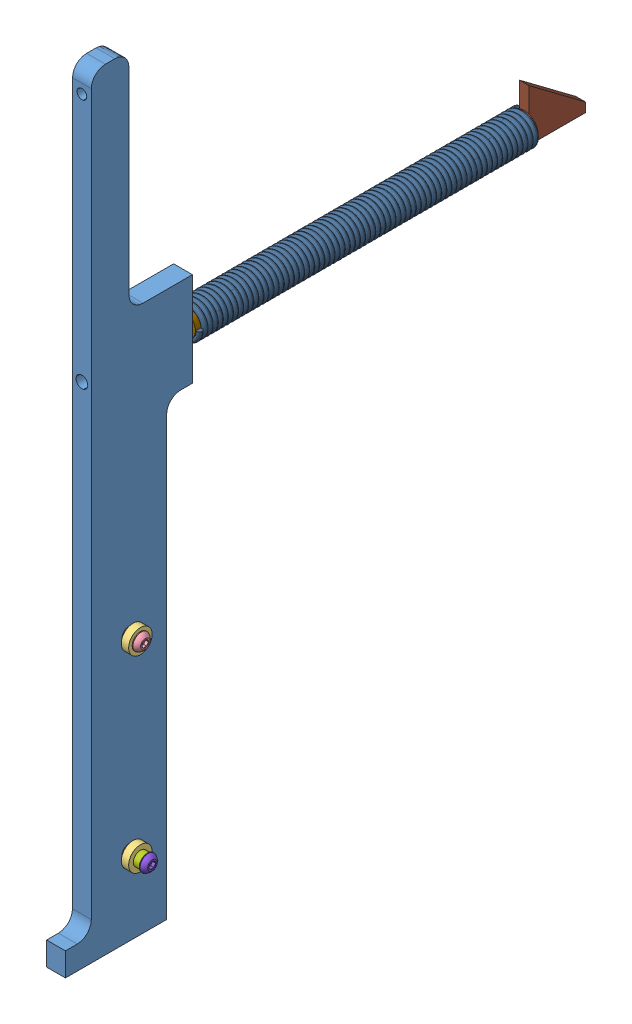
SolidWorks assembly GE-17047_ASM_25_ASM, configuration Default. Lengths in mm.
Overall size (49.23 520.7 354.14).
22 component instances, 11 part files, 0 mates.
Components (placement in the parent):
- GE-17048_24-1: GE-17048_24 [Default] at origin size (12.7 520.7 85.73)
- GE-17051_2-1: GE-17051_2 [Default] at (15.4686 179.3875 0) x (-1 0 0) z (0 0 1) size (2.77 9.53 9.53)
- GE-17051_2-2: GE-17051_2 [Default] at (0 179.3875 0) x (-1 0 0) z (0 0 1) size (2.77 9.53 9.53)
- GE-17050_3-1: GE-17050_3 [Default] at (15.4686 179.3875 0) size (4.98 15.88 15.88)
- GE-17050_3-2: GE-17050_3 [Default] at (-7.747 179.3875 0) size (4.98 15.88 15.88)
- HW-00501_2-1: HW-00501_2 [Default] at (23.7998 179.3875 0) x (0 1 0) z (1 0 0) size (11.17 11.22 39.58)
- HW-00502_2_ASM-1: HW-00502_2_ASM [Default] at (-4.9784 179.3875 0) x (0 1 0) z (0 0 1) size (11.11 5.36 12.83)
  - MANIFOLD_SOLID_BREP_212996-1: MANIFOLD_SOLID_BREP_212996 [Default] at origin size (10.65 1.02 10.65)
  - MANIFOLD_SOLID_BREP_214924-1: MANIFOLD_SOLID_BREP_214924 [Default] at origin size (11.11 5.36 12.83)
- GE-17051_2-3: GE-17051_2 [Default] at (15.4686 52.3875 0) x (-1 0 0) z (0 0 1) size (2.77 9.53 9.53)
- GE-17051_2-4: GE-17051_2 [Default] at (0 52.3875 0) x (-1 0 0) z (0 0 1) size (2.77 9.53 9.53)
- GE-17050_3-3: GE-17050_3 [Default] at (15.4686 52.3875 0) size (4.98 15.88 15.88)
- GE-17050_3-4: GE-17050_3 [Default] at (-7.747 52.3875 0) size (4.98 15.88 15.88)
- GE-17056_5-1: GE-17056_5 [Default] at (20.447 52.3875 0) size (4.76 9.53 9.53)
- GE-17056_5-2: GE-17056_5 [Default] at (-12.5095 52.3875 0) size (4.76 9.53 9.53)
- HW-00502_2_ASM-2: HW-00502_2_ASM [Default] at (-9.7409 52.3875 0) x (0 1 0) z (0 0 1) size (11.11 5.36 12.83)
  - MANIFOLD_SOLID_BREP_212996-1: MANIFOLD_SOLID_BREP_212996 [Default] at origin size (10.65 1.02 10.65)
  - MANIFOLD_SOLID_BREP_214924-1: MANIFOLD_SOLID_BREP_214924 [Default] at origin size (11.11 5.36 12.83)
- HW-00505_3-1: HW-00505_3 [Default] at (28.5623 52.3875 0) x (0 1 0) z (1 0 0) size (11.17 11.22 49.23)
- GE-17061_4-1: GE-17061_4 [Default] at (6.35 336.55 -42.8625) x (0 0 -1) z (0 1 0) size (25.4 16.76 16.76)
- GE-17063_8-1: GE-17063_8 [Default] at (6.35 336.55 -44.577) x (0 -1 0) z (1 0 0) size (24.74 232.22 24.75)
- GE-17064_6-1: GE-17064_6 [Default] at (6.35 336.55 -247.777) x (-1 0 0) z (0 0 -1) size (18.8 34.93 63.5)
